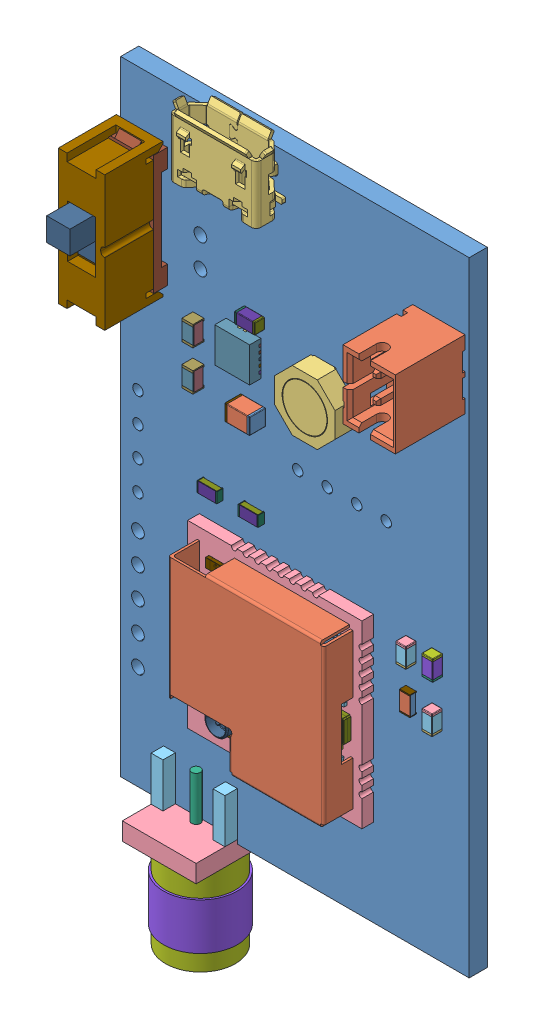
SolidWorks assembly Peggy Receiver, configuration По умолчанию. Lengths in mm.
Overall size (30 63.78 12.1).
247 component instances, 62 part files, 0 mates.
Components (placement in the parent):
- Peggy Receiver.step-1: Peggy Receiver.step [Default] at origin size (30 63.78 12.1)
  - Board.step-1: Board.step [Default] at origin size (30 53.7 1.56)
    - Open CASCADE STEP translator 6.8 1.1.1.step-1: Open CASCADE STEP translator 6.8 1.1.1.step [Default] at (0 0 -1.5596) size (30 53.7 1.56)
  - X3-1.step-1: X3-1.step [Default] at origin size (4.5 5.9 9.4)
    - B2B-PH-K-S(LF)(SN)--3DModel-STEP-56544.step-1: B2B-PH-K-S(LF)(SN)--3DModel-STEP-56544.step [Default] at (27.3908 44.8301 3) x (0 -1 0) z (-1 0 0) size (5.9 9.4 4.5)
  - X2.step-1: X2.step [Default] at origin size (8.07 6.06 3.61)
    - 10103594.step-1: 10103594.step [Default] at (10.4625 50.6099 2.2526) x (1 0 0) z (0 1 0) size (8.07 3.61 6.06)
  - X1.step-1: X1.step [Default] at origin size (6.35 13.15 6.72)
    - 5932012048.step-1: 5932012048.step [Default] at (6.8669 -0.4251 -2.8) size (6.35 1.52 6.35)
      - Extruded.step-1: Extruded.step [Default] at origin size (6.35 1.52 6.35)
    - 5932011648.step-1: 5932011648.step [Default] at (9.5339 2.2419 0) size (1.02 3.81 1.07)
      - Extruded-0.step-1: Extruded-0.step [Default] at origin size (1.02 3.81 1.07)
    - 5932011648.step-2: 5932011648.step [Default] at (4.1999 2.2419 0) size (1.02 3.81 1.07)
      - Extruded-0.step-1: Extruded-0.step [Default] at origin size (1.02 3.81 1.07)
    - 5932011008.step-1: 5932011008.step [Default] at (6.8685 0.3352 0.38) x (-1 0 0) z (0 1 0) size (0.76 0.76 3.81)
      - Cylinder.step-1: Cylinder.step [Default] at origin size (0.76 0.76 3.81)
    - 5932011648.step-3: 5932011648.step [Default] at (9.5339 2.2419 -2.8) size (1.02 3.81 1.07)
      - Extruded-0.step-1: Extruded-0.step [Default] at origin size (1.02 3.81 1.07)
    - 5932011648.step-4: 5932011648.step [Default] at (4.1999 2.2419 -2.8) size (1.02 3.81 1.07)
      - Extruded-0.step-1: Extruded-0.step [Default] at origin size (1.02 3.81 1.07)
    - 5932010128.step-1: 5932010128.step [Default] at (6.867 -9.0051 0) x (-1 0 0) z (0 1 0) size (6 6 7.87)
      - Cylinder-1.step-1: Cylinder-1.step [Default] at origin size (6 6 7.87)
    - 5932009728.step-1: 5932009728.step [Default] at (6.862 -7.5051 0) x (-1 0 0) z (0 1 0) size (6.34 6.34 4)
      - Cylinder-2.step-1: Cylinder-2.step [Default] at origin size (6.34 6.34 4)
  - SW1.step-1: SW1.step [Default] at origin size (4 11.6 12.1)
    - User_Library-EG1218.step-1: User_Library-EG1218.step [Default] at (2.032 43.79 0.4) x (0 -1 0) z (0 0 1) size (11.6 4 12.1)
      - User_Library-EG1218_EG1218_Housing.step-1: User_Library-EG1218_EG1218_Housing.step [Default] at origin size (11.6 4 5)
      - User_Library-EG1218_EG1218_Actuator.step-1: User_Library-EG1218_EG1218_Actuator.step [Default] at (-1.25 0 4.1) size (6.75 2.75 5.75)
      - User_Library-EG1218_EG1218A_Terminals.step-1: User_Library-EG1218_EG1218A_Terminals.step [Default] at (0 0 -0.4) size (11.4 4 7.8)
  - R6.step-1: R6.step [Default] at origin size (0.95 1.75 0.95)
    - 5470717088.step-1: 5470717088.step [Default] at (6.6945 36.9 0) x (0 -1 0) z (0 0 1) size (1.75 0.95 0.95)
      - Terminal.step-1: Terminal.step [Default] at (-0.875 -0.475 0) size (0.2 0.95 0.95)
        - Open_CASCADE_STEP_translator_6.8_13.2.1.step-1: Open_CASCADE_STEP_translator_6.8_13.2.1.step [Default] at origin size (0.2 0.95 0.95)
      - Terminal.step-2: Terminal.step [Default] at (0.875 0.475 0) x (-1 0 0) z (0 0 1) size (0.2 0.95 0.95)
        - Open_CASCADE_STEP_translator_6.8_13.2.1.step-1: Open_CASCADE_STEP_translator_6.8_13.2.1.step [Default] at origin size (0.2 0.95 0.95)
      - Mid_Body.step-1: Mid_Body.step [Default] at (-0.875 -0.475 0) size (1.56 0.95 0.76)
      - Mark.step-1: Mark.step [Default] at (-0.675 -0.475 0.855) size (1.35 0.95 0.1)
  - R5.step-1: R5.step [Default] at origin size (0.95 1.75 0.95)
    - 5470717088.step-1: 5470717088.step [Default] at (6.6945 33.4502 0) x (0 -1 0) z (0 0 1) size (1.75 0.95 0.95)
      - Terminal.step-1: Terminal.step [Default] at (-0.875 -0.475 0) size (0.2 0.95 0.95)
        - Open_CASCADE_STEP_translator_6.8_13.2.1.step-1: Open_CASCADE_STEP_translator_6.8_13.2.1.step [Default] at origin size (0.2 0.95 0.95)
      - Terminal.step-2: Terminal.step [Default] at (0.875 0.475 0) x (-1 0 0) z (0 0 1) size (0.2 0.95 0.95)
        - Open_CASCADE_STEP_translator_6.8_13.2.1.step-1: Open_CASCADE_STEP_translator_6.8_13.2.1.step [Default] at origin size (0.2 0.95 0.95)
      - Mid_Body.step-1: Mid_Body.step [Default] at (-0.875 -0.475 0) size (1.56 0.95 0.76)
      - Mark.step-1: Mark.step [Default] at (-0.675 -0.475 0.855) size (1.35 0.95 0.1)
  - R4.step-1: R4.step [Default] at origin size (1.7 0.9 0.55)
    - 5470718048.step-1: 5470718048.step [Default] at (7.9751 25.4751 0) size (1.7 0.9 0.55)
      - Terminal-1.step-1: Terminal-1.step [Default] at (-0.85 -0.45 0) size (0.1 0.9 0.55)
        - Open_CASCADE_STEP_translator_6.8_15.2.1.step-1: Open_CASCADE_STEP_translator_6.8_15.2.1.step [Default] at origin size (0.1 0.9 0.55)
      - Terminal-1.step-2: Terminal-1.step [Default] at (0.85 0.45 0) x (-1 0 0) z (0 0 1) size (0.1 0.9 0.55)
        - Open_CASCADE_STEP_translator_6.8_15.2.1.step-1: Open_CASCADE_STEP_translator_6.8_15.2.1.step [Default] at origin size (0.1 0.9 0.55)
      - Mid_Body-3.step-1: Mid_Body-3.step [Default] at (-0.85 -0.45 0) size (1.59 0.9 0.44)
      - Mark-4.step-1: Mark-4.step [Default] at (-0.75 -0.45 0.495) size (1.5 0.9 0.06)
  - R3.step-1: R3.step [Default] at origin size (1.7 0.9 0.55)
    - 5470718048.step-1: 5470718048.step [Default] at (11.517 25.4832 0) size (1.7 0.9 0.55)
      - Terminal-1.step-1: Terminal-1.step [Default] at (-0.85 -0.45 0) size (0.1 0.9 0.55)
        - Open_CASCADE_STEP_translator_6.8_15.2.1.step-1: Open_CASCADE_STEP_translator_6.8_15.2.1.step [Default] at origin size (0.1 0.9 0.55)
      - Terminal-1.step-2: Terminal-1.step [Default] at (0.85 0.45 0) x (-1 0 0) z (0 0 1) size (0.1 0.9 0.55)
        - Open_CASCADE_STEP_translator_6.8_15.2.1.step-1: Open_CASCADE_STEP_translator_6.8_15.2.1.step [Default] at origin size (0.1 0.9 0.55)
      - Mid_Body-3.step-1: Mid_Body-3.step [Default] at (-0.85 -0.45 0) size (1.59 0.9 0.44)
      - Mark-4.step-1: Mark-4.step [Default] at (-0.75 -0.45 0.495) size (1.5 0.9 0.06)
  - R1.step-1: R1.step [Default] at origin size (0.9 1.7 0.55)
    - 5470716128.step-1: 5470716128.step [Default] at (24.9999 18.2501 0) x (0 1 0) z (0 0 1) size (1.7 0.9 0.55)
      - Terminal-2.step-1: Terminal-2.step [Default] at (-0.85 -0.45 0) size (0.1 0.9 0.55)
        - Open_CASCADE_STEP_translator_6.8_15.2.1-5.step-1: Open_CASCADE_STEP_translator_6.8_15.2.1-5.step [Default] at origin size (0.1 0.9 0.55)
      - Terminal-2.step-2: Terminal-2.step [Default] at (0.85 0.45 0) x (-1 0 0) z (0 0 1) size (0.1 0.9 0.55)
        - Open_CASCADE_STEP_translator_6.8_15.2.1-5.step-1: Open_CASCADE_STEP_translator_6.8_15.2.1-5.step [Default] at origin size (0.1 0.9 0.55)
      - Mid_Body-6.step-1: Mid_Body-6.step [Default] at (-0.85 -0.45 0) size (1.59 0.9 0.44)
      - Mark-7.step-1: Mark-7.step [Default] at (-0.75 -0.45 0.495) size (1.5 0.9 0.06)
  - L1.step-1: L1.step [Default] at origin size (5.2 5.2 1.8)
    - 5470723008.step-1: 5470723008.step [Default] at (17.65 37.25 0.2) x (0 1 0) z (1 0 0) size (5.2 1.8 5.2)
  - DD2.step-1: DD2.step [Default] at origin size (15 15.5 3.52)
    - 3D_RAK3172.step-1: 3D_RAK3172.step [Default] at (21.767 23.0001 1) x (-1 0 0) z (0 0 1) size (15 15.5 3.52)
      - Board-1.step-1: Board-1.step [Default] at origin size (15 15.5 1.01)
        - Open_CASCADE_STEP_translator_6.8_1.1.1.step-1: Open_CASCADE_STEP_translator_6.8_1.1.1.step [Default] at (0 0 -1.014) size (15 15.5 1.01)
          - Open_CASCADE_STEP_translator_6.8_1.1.1.1.step-1: Open_CASCADE_STEP_translator_6.8_1.1.1.1.step [Default] at origin size (15 15.5 1.01)
      - R11.step-1: R11.step [Default] at origin size (0.6 0.3 0.3)
        - 0201_SMD_Capacitor.step-1: 0201_SMD_Capacitor.step [Default] at (3.4751 6.9342 0.2794) x (-1 0 0) z (0 0 1) size (0.6 0.3 0.3)
      - U2.step-1: U2.step [Default] at origin size (0.99 1.02 0.75)
        - 6590464912.step-1: 6590464912.step [Default] at (5.4483 13.05 0) size (0.99 1.02 0.75)
          - Extruded-8.step-1: Extruded-8.step [Default] at origin size (0.99 1.02 0.75)
      - R4-1.step-1: R4-1.step [Default] at origin size (0.68 0.33 0.34)
        - R0201.step-1: R0201.step [Default] at (3.9176 5.9192 0) x (1 0 0) z (0 -1 0) size (0.68 0.34 0.33)
      - R3-1.step-1: R3-1.step [Default] at origin size (0.33 0.68 0.34)
        - R0201.step-1: R0201.step [Default] at (4.1676 5.6692 0) x (0 1 0) z (1 0 0) size (0.68 0.34 0.33)
      - L2.step-1: L2.step [Default] at origin size (1.15 0.55 0.41)
        - RES_1005-0402.step-1: RES_1005-0402.step [Default] at (2.2661 6.0198 0) x (1 0 0) z (0 -1 0) size (1.15 0.41 0.55)
      - C10.step-1: C10.step [Default] at origin size (0.6 0.3 0.3)
        - 0201_SMD_Capacitor.step-1: 0201_SMD_Capacitor.step [Default] at (7.1835 13.462 0.2794) x (-1 0 0) z (0 0 1) size (0.6 0.3 0.3)
      - C9.step-1: C9.step [Default] at origin size (0.6 0.3 0.3)
        - 0201_SMD_Capacitor.step-1: 0201_SMD_Capacitor.step [Default] at (7.1835 13.97 0.2794) x (-1 0 0) z (0 0 1) size (0.6 0.3 0.3)
      - C8.step-1: C8.step [Default] at origin size (0.6 0.3 0.3)
        - 0201_SMD_Capacitor.step-1: 0201_SMD_Capacitor.step [Default] at (7.1835 12.954 0.2794) x (-1 0 0) z (0 0 1) size (0.6 0.3 0.3)
      - C7.step-1: C7.step [Default] at origin size (0.6 0.3 0.3)
        - 0201_SMD_Capacitor.step-1: 0201_SMD_Capacitor.step [Default] at (6.0793 11.938 0.2794) x (1 0 0) z (0 0 1) size (0.6 0.3 0.3)
      - C6.step-1: C6.step [Default] at origin size (0.6 0.3 0.3)
        - 0201_SMD_Capacitor.step-1: 0201_SMD_Capacitor.step [Default] at (3.8855 13.5541 0.2794) x (-1 0 0) z (0 0 1) size (0.6 0.3 0.3)
      - CON1.step-1: CON1.step [Default] at origin size (3.4 3.1 1.25)
        - UFL-R-SMD.step-1: UFL-R-SMD.step [Default] at (11.3537 12.7757 0) x (1 0 0) z (0 0 1) size (3.4 3.1 1.25)
          - Part_525.step-1: Part_525.step [Default] at origin size (3 2.6 0.35)
          - Part_739.step-1: Part_739.step [Default] at origin size (2 2 0.9)
          - Part_578.step-1: Part_578.step [Default] at origin size (0.6 0.5 0.1)
          - Part_540.step-1: Part_540.step [Default] at origin size (0.4 1.8 0.1)
          - Part_562.step-1: Part_562.step [Default] at origin size (0.4 1.8 0.1)
          - Part_555.step-1: Part_555.step [Default] at origin size (0.6 0.5 0.1)
      - C4.step-1: C4.step [Default] at origin size (0.6 0.3 0.3)
        - 0201_SMD_Capacitor.step-1: 0201_SMD_Capacitor.step [Default] at (3.7799 9.398 0.2794) x (-1 0 0) z (0 0 1) size (0.6 0.3 0.3)
      - U1.step-1: U1.step [Default] at origin size (7.02 7.02 0.8)
        - QFN48_7x7.step-1: QFN48_7x7.step [Default] at (8.8366 6.9818 0) x (0 1 0) z (1 0 0) size (7.02 0.8 7.02)
      - X1-1.step-1: X1-1.step [Default] at origin size (1.61 2.01 0.71)
        - NT2016SA.step-1: NT2016SA.step [Default] at (1.7496 8.4946 0) x (0 1 0) z (1 0 0) size (2.01 0.71 1.61)
      - C43.step-1: C43.step [Default] at origin size (0.6 0.3 0.3)
        - 0201_SMD_Capacitor.step-1: 0201_SMD_Capacitor.step [Default] at (3.7799 9.9822 0.2794) x (-1 0 0) z (0 0 1) size (0.6 0.3 0.3)
      - C42.step-1: C42.step [Default] at origin size (0.3 0.6 0.3)
        - 0201_SMD_Capacitor.step-1: 0201_SMD_Capacitor.step [Default] at (3.0734 7.9709 0.2794) x (0 -1 0) z (0 0 1) size (0.6 0.3 0.3)
      - R9.step-1: R9.step [Default] at origin size (0.6 0.3 0.3)
        - 0201_SMD_Capacitor.step-1: 0201_SMD_Capacitor.step [Default] at (3.7799 8.8138 0.2794) x (-1 0 0) z (0 0 1) size (0.6 0.3 0.3)
      - C1.step-1: C1.step [Default] at origin size (0.6 0.3 0.3)
        - 0201_SMD_Capacitor.step-1: 0201_SMD_Capacitor.step [Default] at (7.0445 11.557 0.2794) x (1 0 0) z (0 0 1) size (0.6 0.3 0.3)
      - C2.step-1: C2.step [Default] at origin size (0.3 0.6 0.3)
        - 0201_SMD_Capacitor.step-1: 0201_SMD_Capacitor.step [Default] at (7.9756 12.2635 0.2794) x (0 -1 0) z (0 0 1) size (0.6 0.3 0.3)
      - C3.step-1: C3.step [Default] at origin size (0.3 0.6 0.3)
        - 0201_SMD_Capacitor.step-1: 0201_SMD_Capacitor.step [Default] at (2.1844 13.4518 0.2794) x (0 -1 0) z (0 0 1) size (0.6 0.3 0.3)
      - C11.step-1: C11.step [Default] at origin size (0.6 0.3 0.3)
        - 0201_SMD_Capacitor.step-1: 0201_SMD_Capacitor.step [Default] at (1.6623 11.9866 0.2794) x (1 0 0) z (0 0 1) size (0.6 0.3 0.3)
      - C12.step-1: C12.step [Default] at origin size (0.6 0.3 0.3)
        - 0201_SMD_Capacitor.step-1: 0201_SMD_Capacitor.step [Default] at (3.2813 12.573 0.2794) x (1 0 0) z (0 0 1) size (0.6 0.3 0.3)
      - C13.step-1: C13.step [Default] at origin size (0.3 0.6 0.3)
        - 0201_SMD_Capacitor.step-1: 0201_SMD_Capacitor.step [Default] at (4.4958 12.0697 0.2794) x (0 1 0) z (0 0 1) size (0.6 0.3 0.3)
      - C14.step-1: C14.step [Default] at origin size (0.3 0.6 0.3)
        - 0201_SMD_Capacitor.step-1: 0201_SMD_Capacitor.step [Default] at (2.7178 12.6739 0.2794) x (0 -1 0) z (0 0 1) size (0.6 0.3 0.3)
      - C17.step-1: C17.step [Default] at origin size (0.3 0.6 0.3)
        - 0201_SMD_Capacitor.step-1: 0201_SMD_Capacitor.step [Default] at (7.6708 14.4693 0.2794) x (0 -1 0) z (0 0 1) size (0.6 0.3 0.3)
      - C18.step-1: C18.step [Default] at origin size (0.6 0.3 0.3)
        - 0201_SMD_Capacitor.step-1: 0201_SMD_Capacitor.step [Default] at (9.1901 14.1224 0.2794) x (-1 0 0) z (0 0 1) size (0.6 0.3 0.3)
      - C19.step-1: C19.step [Default] at origin size (0.3 0.6 0.3)
        - 0201_SMD_Capacitor.step-1: 0201_SMD_Capacitor.step [Default] at (2.8814 10.8799 0.2794) x (0 1 0) z (0 0 1) size (0.6 0.3 0.3)
      - C22.step-1: C22.step [Default] at origin size (0.3 0.6 0.3)
        - 0201_SMD_Capacitor.step-1: 0201_SMD_Capacitor.step [Default] at (2.0432 11.4801 0.2794) x (0 -1 0) z (0 0 1) size (0.6 0.3 0.3)
      - C21.step-1: C21.step [Default] at origin size (0.3 0.6 0.3)
        - 0201_SMD_Capacitor.step-1: 0201_SMD_Capacitor.step [Default] at (1.5606 11.4801 0.2794) x (0 -1 0) z (0 0 1) size (0.6 0.3 0.3)
      - C23.step-1: C23.step [Default] at origin size (1 0.5 0.5)
        - C0402.step-1: C0402.step [Default] at (8.9644 1.5539 0.254) x (1 0 0) z (0 0 1) size (1 0.5 0.5)
      - C24.step-1: C24.step [Default] at origin size (0.6 0.3 0.3)
        - 0201_SMD_Capacitor.step-1: 0201_SMD_Capacitor.step [Default] at (4.7197 3.8862 0.2794) x (-1 0 0) z (0 0 1) size (0.6 0.3 0.3)
      - C26.step-1: C26.step [Default] at origin size (0.3 0.6 0.3)
        - 0201_SMD_Capacitor.step-1: 0201_SMD_Capacitor.step [Default] at (10.541 2.2265 0.2794) x (0 -1 0) z (0 0 1) size (0.6 0.3 0.3)
      - C44.step-1: C44.step [Default] at origin size (0.6 0.3 0.3)
        - 0201_SMD_Capacitor.step-1: 0201_SMD_Capacitor.step [Default] at (4.7919 9.9822 0.2794) x (-1 0 0) z (0 0 1) size (0.6 0.3 0.3)
      - C29.step-1: C29.step [Default] at origin size (0.6 0.3 0.3)
        - 0201_SMD_Capacitor.step-1: 0201_SMD_Capacitor.step [Default] at (3.9925 7.8486 0.2794) x (1 0 0) z (0 0 1) size (0.6 0.3 0.3)
      - C25.step-1: C25.step [Default] at origin size (0.3 0.6 0.3)
        - 0201_SMD_Capacitor.step-1: 0201_SMD_Capacitor.step [Default] at (10.287 1.6263 0.2794) x (0 1 0) z (0 0 1) size (0.6 0.3 0.3)
      - C31.step-1: C31.step [Default] at origin size (0.6 0.3 0.3)
        - 0201_SMD_Capacitor.step-1: 0201_SMD_Capacitor.step [Default] at (3.9965 7.239 0.2794) x (1 0 0) z (0 0 1) size (0.6 0.3 0.3)
      - C32.step-1: C32.step [Default] at origin size (0.6 0.3 0.3)
        - 0201_SMD_Capacitor.step-1: 0201_SMD_Capacitor.step [Default] at (7.8533 2.3622 0.2794) x (1 0 0) z (0 0 1) size (0.6 0.3 0.3)
      - C33.step-1: C33.step [Default] at origin size (1 0.5 0.5)
        - C0402.step-1: C0402.step [Default] at (5.3048 2.0461 0.254) x (-1 0 0) z (0 0 1) size (1 0.5 0.5)
      - C34.step-1: C34.step [Default] at origin size (0.3 0.6 0.3)
        - 0201_SMD_Capacitor.step-1: 0201_SMD_Capacitor.step [Default] at (4.318 4.2211 0.2794) x (0 1 0) z (0 0 1) size (0.6 0.3 0.3)
      - C35.step-1: C35.step [Default] at origin size (0.6 0.3 0.3)
        - 0201_SMD_Capacitor.step-1: 0201_SMD_Capacitor.step [Default] at (9.0365 2.3622 0.2794) x (1 0 0) z (0 0 1) size (0.6 0.3 0.3)
      - C36.step-1: C36.step [Default] at origin size (0.3 0.6 0.3)
        - 0201_SMD_Capacitor.step-1: 0201_SMD_Capacitor.step [Default] at (13.0302 10.0751 0.2794) x (0 -1 0) z (0 0 1) size (0.6 0.3 0.3)
      - C37.step-1: C37.step [Default] at origin size (0.3 0.6 0.3)
        - 0201_SMD_Capacitor.step-1: 0201_SMD_Capacitor.step [Default] at (3.7338 4.2211 0.2794) x (0 1 0) z (0 0 1) size (0.6 0.3 0.3)
      - C38.step-1: C38.step [Default] at origin size (1 0.5 0.5)
        - C0402.step-1: C0402.step [Default] at (2.3114 4.7323 0.254) x (1 0 0) z (0 0 1) size (1 0.5 0.5)
      - C39.step-1: C39.step [Default] at origin size (0.6 0.3 0.3)
        - 0201_SMD_Capacitor.step-1: 0201_SMD_Capacitor.step [Default] at (4.0593 3.1881 0.2794) x (-1 0 0) z (0 0 1) size (0.6 0.3 0.3)
      - C40.step-1: C40.step [Default] at origin size (0.3 0.6 0.3)
        - 0201_SMD_Capacitor.step-1: 0201_SMD_Capacitor.step [Default] at (3.6576 1.7319 0.2794) x (0 1 0) z (0 0 1) size (0.6 0.3 0.3)
      - L1-1.step-1: L1-1.step [Default] at origin size (0.68 0.33 0.34)
        - R0201.step-1: R0201.step [Default] at (7.8526 11.2014 0) x (-1 0 0) z (0 1 0) size (0.68 0.34 0.33)
      - L3.step-1: L3.step [Default] at origin size (0.33 0.68 0.34)
        - R0201.step-1: R0201.step [Default] at (1.7272 13.1318 0) x (0 -1 0) z (-1 0 0) size (0.68 0.34 0.33)
      - L5.step-1: L5.step [Default] at origin size (0.68 0.33 0.34)
        - R0201.step-1: R0201.step [Default] at (8.0772 13.3096 0) x (-1 0 0) z (0 1 0) size (0.68 0.34 0.33)
      - L6.step-1: L6.step [Default] at origin size (1 0.5 0.5)
        - C0402.step-1: C0402.step [Default] at (5.822 11.0823 0.254) x (1 0 0) z (0 0 1) size (1 0.5 0.5)
      - L7.step-1: L7.step [Default] at origin size (0.68 0.33 0.34)
        - R0201.step-1: R0201.step [Default] at (3.5854 12.1158 0) x (1 0 0) z (0 -1 0) size (0.68 0.34 0.33)
      - L9.step-1: L9.step [Default] at origin size (1.15 0.55 0.41)
        - RES_1005-0402.step-1: RES_1005-0402.step [Default] at (3.9641 11.3538 0) x (-1 0 0) z (0 1 0) size (1.15 0.41 0.55)
      - L20.step-1: L20.step [Default] at origin size (1.6 0.8 0.3)
        - 6559637360.step-1: 6559637360.step [Default] at (12.3698 2.0828 0) x (-1 0 0) z (0 1 0) size (1.6 0.3 0.8)
      - L30.step-1: L30.step [Default] at origin size (1.15 0.55 0.41)
        - RES_1005-0402.step-1: RES_1005-0402.step [Default] at (7.1263 1.8 0) x (-1 0 0) z (0 1 0) size (1.15 0.41 0.55)
      - X2-1.step-1: X2-1.step [Default] at origin size (1.2 2 0.61)
        - crystal_rtf2012.step-1: crystal_rtf2012.step [Default] at (2.25 2.8402 0) x (0 1 0) z (1 0 0) size (2 0.61 1.2)
      - R2.step-1: R2.step [Default] at origin size (0.68 0.33 0.34)
        - R0201.step-1: R0201.step [Default] at (1.9613 10.1854 0) x (1 0 0) z (0 -1 0) size (0.68 0.34 0.33)
      - C5.step-1: C5.step [Default] at origin size (0.6 0.3 0.3)
        - 0201_SMD_Capacitor.step-1: 0201_SMD_Capacitor.step [Default] at (1.8749 6.9342 0.2794) x (-1 0 0) z (0 0 1) size (0.6 0.3 0.3)
      - Free-Models.step-1: Free-Models.step [Default] at origin size (13.4 13.9 2.5)
        - D030A-______.step-1: D030A-______.step [Default] at (2.429 -1.8288 0) size (13.4 13.9 2.5)
  - DA1.step-1: DA1.step [Default] at origin size (3 3 1)
    - 5470722288.step-1: 5470722288.step [Default] at (10.6 37.25 0) x (-1 0 0) z (0 0 1) size (3 3 1)
      - FRAME-DRC0010J.step-1: FRAME-DRC0010J.step [Default] x (1 0 0) z (0 -1 0) size (3 0.2 3)
        - Open CASCADE STEP translator 6.8 1.13.1.2.1.step-1: Open CASCADE STEP translator 6.8 1.13.1.2.1.step [Default] at origin size (1.9 0.2 3)
        - Open CASCADE STEP translator 6.8 1.13.1.2.2.step-1: Open CASCADE STEP translator 6.8 1.13.1.2.2.step [Default] at origin size (0.4 0.2 0.24)
        - Open CASCADE STEP translator 6.8 1.13.1.2.3.step-1: Open CASCADE STEP translator 6.8 1.13.1.2.3.step [Default] at origin size (0.4 0.2 0.24)
        - Open CASCADE STEP translator 6.8 1.13.1.2.4.step-1: Open CASCADE STEP translator 6.8 1.13.1.2.4.step [Default] at origin size (0.4 0.2 0.24)
        - Open CASCADE STEP translator 6.8 1.13.1.2.5.step-1: Open CASCADE STEP translator 6.8 1.13.1.2.5.step [Default] at origin size (0.4 0.2 0.24)
        - Open CASCADE STEP translator 6.8 1.13.1.2.6.step-1: Open CASCADE STEP translator 6.8 1.13.1.2.6.step [Default] at origin size (0.4 0.2 0.24)
        - Open CASCADE STEP translator 6.8 1.13.1.2.7.step-1: Open CASCADE STEP translator 6.8 1.13.1.2.7.step [Default] at origin size (0.4 0.2 0.24)
        - Open CASCADE STEP translator 6.8 1.13.1.2.8.step-1: Open CASCADE STEP translator 6.8 1.13.1.2.8.step [Default] at origin size (0.4 0.2 0.24)
        - Open CASCADE STEP translator 6.8 1.13.1.2.9.step-1: Open CASCADE STEP translator 6.8 1.13.1.2.9.step [Default] at origin size (0.4 0.2 0.24)
        - Open CASCADE STEP translator 6.8 1.13.1.2.10.step-1: Open CASCADE STEP translator 6.8 1.13.1.2.10.step [Default] at origin size (0.4 0.2 0.24)
        - Open CASCADE STEP translator 6.8 1.13.1.2.11.step-1: Open CASCADE STEP translator 6.8 1.13.1.2.11.step [Default] at origin size (0.4 0.2 0.24)
      - BODY-SON.step-1: BODY-SON.step [Default] at (0 0 0.025) x (1 0 0) z (0 -1 0) size (3 0.97 3)
  - C5-1.step-1: C5-1.step [Default] at origin size (1.75 0.95 0.87)
    - 5470806048.step-1: 5470806048.step [Default] at (11.525 40 0) x (1 0 0) z (0 0 1) size (1.75 0.95 0.87)
      - Terminal-3.step-1: Terminal-3.step [Default] at (-0.875 -0.475 0) size (1.75 0.95 0.87)
        - Open_CASCADE_STEP_translator_6.8_129.1.1.step-1: Open_CASCADE_STEP_translator_6.8_129.1.1.step [Default] at origin size (0.2 0.95 0.87)
        - Open_CASCADE_STEP_translator_6.8_129.1.2.step-1: Open_CASCADE_STEP_translator_6.8_129.1.2.step [Default] at origin size (0.2 0.95 0.87)
      - Mid_Body-9.step-1: Mid_Body-9.step [Default] at (-0.875 -0.475 0) size (1.35 0.95 0.87)
        - Open_CASCADE_STEP_translator_6.8_129.2.1.step-1: Open_CASCADE_STEP_translator_6.8_129.2.1.step [Default] at origin size (1.35 0.95 0.87)
  - C4-1.step-1: C4-1.step [Default] at origin size (2.15 1.4 1.4)
    - 5470717888.step-1: 5470717888.step [Default] at (11.4126 33.0502 0) size (2.15 1.4 1.4)
      - Terminal-4.step-1: Terminal-4.step [Default] at (-1.075 -0.7 0) size (2.15 1.4 1.4)
        - Open_CASCADE_STEP_translator_6.8_5.1.1.step-1: Open_CASCADE_STEP_translator_6.8_5.1.1.step [Default] at origin size (0.2 1.4 1.4)
        - Open_CASCADE_STEP_translator_6.8_5.1.2.step-1: Open_CASCADE_STEP_translator_6.8_5.1.2.step [Default] at origin size (0.2 1.4 1.4)
      - Mid_Body-1.step-1: Mid_Body-1.step [Default] at (-1.075 -0.7 0) size (1.75 1.4 1.4)
        - Open_CASCADE_STEP_translator_6.8_5.2.1.step-1: Open_CASCADE_STEP_translator_6.8_5.2.1.step [Default] at origin size (1.75 1.4 1.4)
  - C3-1.step-1: C3-1.step [Default] at origin size (0.9 1.7 0.9)
    - 5470730768.step-1: 5470730768.step [Default] at (27.25 18.1 0) x (0 1 0) z (0 0 1) size (1.7 0.9 0.9)
      - Terminal-5.step-1: Terminal-5.step [Default] at (-0.85 -0.45 0) size (1.7 0.9 0.9)
        - Open_CASCADE_STEP_translator_6.8_2.1.1.step-1: Open_CASCADE_STEP_translator_6.8_2.1.1.step [Default] at origin size (0.2 0.9 0.9)
        - Open_CASCADE_STEP_translator_6.8_2.1.2.step-1: Open_CASCADE_STEP_translator_6.8_2.1.2.step [Default] at origin size (0.2 0.9 0.9)
      - Mid_Body-2.step-1: Mid_Body-2.step [Default] at (-0.85 -0.45 0) size (1.3 0.9 0.9)
        - Open_CASCADE_STEP_translator_6.8_2.2.1.step-1: Open_CASCADE_STEP_translator_6.8_2.2.1.step [Default] at origin size (1.3 0.9 0.9)
  - C2-1.step-1: C2-1.step [Default] at origin size (0.95 1.75 0.87)
    - 5470730288.step-1: 5470730288.step [Default] at (27.25 22.175 0) x (0 1 0) z (0 0 1) size (1.75 0.95 0.87)
      - Terminal-6.step-1: Terminal-6.step [Default] at (-0.875 -0.475 0) size (1.75 0.95 0.87)
        - Open_CASCADE_STEP_translator_6.8_129.1.1-10.step-1: Open_CASCADE_STEP_translator_6.8_129.1.1-10.step [Default] at origin size (0.2 0.95 0.87)
        - Open_CASCADE_STEP_translator_6.8_129.1.2-11.step-1: Open_CASCADE_STEP_translator_6.8_129.1.2-11.step [Default] at origin size (0.2 0.95 0.87)
      - Mid_Body-3-12.step-1: Mid_Body-3-12.step [Default] at (-0.875 -0.475 0) size (1.35 0.95 0.87)
        - Open_CASCADE_STEP_translator_6.8_129.2.1-13.step-1: Open_CASCADE_STEP_translator_6.8_129.2.1-13.step [Default] at origin size (1.35 0.95 0.87)
  - C1-1.step-1: C1-1.step [Default] at origin size (0.9 1.7 0.9)
    - 5470730768.step-1: 5470730768.step [Default] at (25 22 0) x (0 1 0) z (0 0 1) size (1.7 0.9 0.9)
      - Terminal-5.step-1: Terminal-5.step [Default] at (-0.85 -0.45 0) size (1.7 0.9 0.9)
        - Open_CASCADE_STEP_translator_6.8_2.1.1.step-1: Open_CASCADE_STEP_translator_6.8_2.1.1.step [Default] at origin size (0.2 0.9 0.9)
        - Open_CASCADE_STEP_translator_6.8_2.1.2.step-1: Open_CASCADE_STEP_translator_6.8_2.1.2.step [Default] at origin size (0.2 0.9 0.9)
      - Mid_Body-2.step-1: Mid_Body-2.step [Default] at (-0.85 -0.45 0) size (1.3 0.9 0.9)
        - Open_CASCADE_STEP_translator_6.8_2.2.1.step-1: Open_CASCADE_STEP_translator_6.8_2.2.1.step [Default] at origin size (1.3 0.9 0.9)
